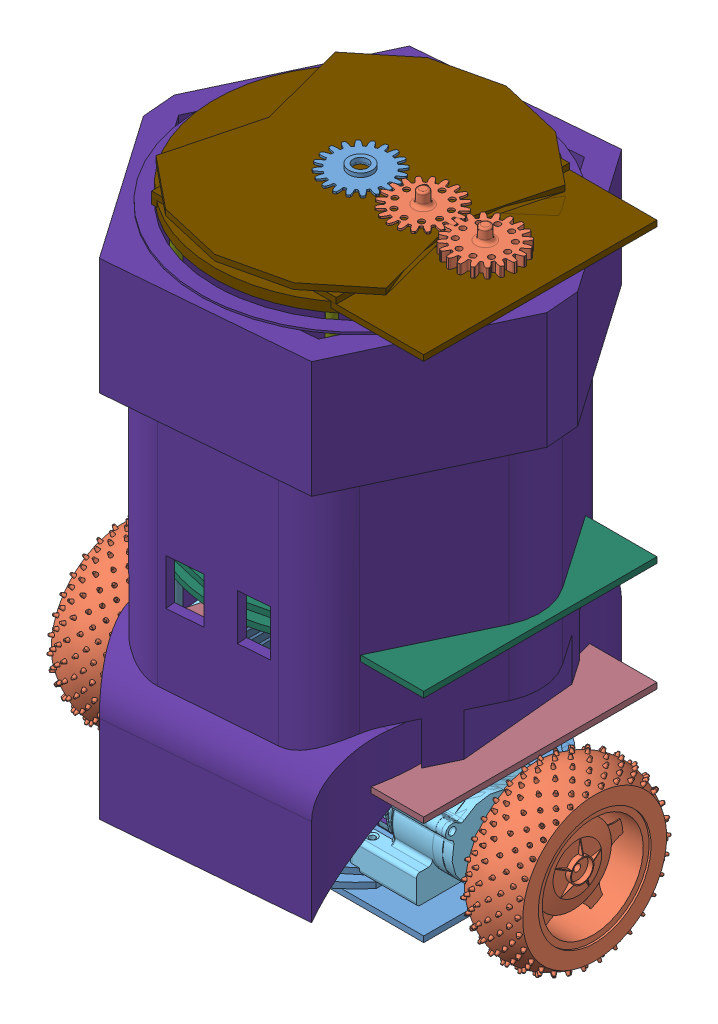
SolidWorks assembly Assembly_2, configuration Default. Lengths in mm.
Overall size (242.54 323.12 157.59).
45 component instances, 20 part files, 99 mates.
Components (placement in the parent):
- BASE PLATE COMPACT-1: BASE PLATE COMPACT [Default] at (9.1956 73.2306 176.3525) size (151.66 9 157.59)
- 85mm_Wheel-1: 85mm_Wheel [Default] at (-49.5434 86.804 117.1986) x (0 0.469219 0.883082) z (0 -0.883082 0.469219) size (89.76 30.03 89.76)
- Bearing_large-1: Bearing_large [Default] at (149.0346 86.804 117.1064) x (0 0.302035 0.953297) z (-1 0 0) size (34 34 10)
- Bearing_Modifiable-1: Bearing_Modifiable [Default] at (-9.2134 86.804 117.1986) x (0 0 -1) z (1 0 0) size (16 16 5)
- Gear Box Covering - Modifiable-1: Gear Box Covering - Modifiable [Default] at (122.6046 86.804 117.1064) x (0 -0.541121 -0.840945) z (1 0 0) size (87.3 57.46 46.55)
- Gear_Driven - LARGE-1: Gear_Driven - LARGE [Default] at (132.5346 86.804 117.1064) x (0 -0.920513 -0.390712) z (1 0 0) size (41.92 41.92 47.93)
- Gear_Driver-1: Gear_Driver [Default] at (129.4046 103.2 142.587) x (0 0.064546 -0.997915) z (1 0 0) size (21.81 21.81 25.3)
- IG32 MOTORS-1: IG32 MOTORS [Default] at (112.6046 103.2 142.587) x (-1 0 0) z (0 0 1) size (92 51.5 40)
- LINE SENSOR-1: LINE SENSOR [Default] at (106.6956 76.2306 130.3525) x (-1 0 0) z (0 0 1) size (100 13.5 28)
- Motor Driver-1: Motor Driver [Default] at (55.9629 132.2306 73.8421) size (71 27 36.5)
- Motor_Main_Shaft-1: Motor_Main_Shaft [Default] at (112.6046 103.2 142.587) x (0 -0.924225 0.381849) z (1 0 0) size (6 6 15)
- Gear Box Covering - Modifiable-2: Gear Box Covering - Modifiable [Default] at (-9.2134 86.804 117.1986) x (0 -0.541121 0.840945) z (-1 0 0) size (87.3 57.46 46.55)
- IG32 MOTORS-2: IG32 MOTORS [Default] at (0.7866 103.2 91.718) size (92 51.5 40)
- Motor_Main_Shaft-2: Motor_Main_Shaft [Default] at (-14.2134 103.2 91.718) x (0 0 -1) z (1 0 0) size (6 6 15)
- Gear_Driver-2: Gear_Driver [Default] at (-16.0134 103.2 91.718) x (0 0.135257 0.99081) z (-1 0 0) size (21.81 21.81 25.3)
- Gear_Driven - LARGE-2: Gear_Driven - LARGE [Default] at (-19.1434 86.804 117.1986) x (0 0.469219 0.883082) z (-1 0 0) size (41.92 41.92 47.93)
- Bearing_Modifiable-2: Bearing_Modifiable [Default] at (139.0346 103.2 142.587) x (0 -0.922949 -0.384923) z (1 0 0) size (16 16 5)
- Bearing_Modifiable-3: Bearing_Modifiable [Default] at (-30.6434 103.2 91.718) x (0 0.129255 -0.991611) z (1 0 0) size (16 16 5)
- Bearing_Modifiable-4: Bearing_Modifiable [Default] at (122.6046 86.804 117.1064) x (0 0.011286 0.999936) z (-1 0 0) size (16 16 5)
- Bearing_large-2: Bearing_large [Default] at (-35.6434 86.804 117.1986) x (0 0 -1) z (1 0 0) size (34 34 10)
- 85mm_Wheel-2: 85mm_Wheel [Default] at (162.9346 86.804 117.1064) x (0 -0.12189 -0.992544) z (0 -0.992544 0.12189) size (89.76 30.03 89.76)
- 4cm_spacers-1: 4cm_spacers [Default] at (96.6956 129.2306 61.5025) x (0.827993 0 0.560738) z (0 -1 0) size (5 5 55)
- 4cm_spacers-2: 4cm_spacers [Default] at (96.6956 129.2306 171.2025) x (0.889434 0 0.457064) z (0 -1 0) size (5 5 55)
- 4cm_spacers-3: 4cm_spacers [Default] at (16.6956 129.2306 171.2025) x (0.138561 0 0.990354) z (0 -1 0) size (5 5 55)
- 4cm_spacers-4: 4cm_spacers [Default] at (16.6956 129.2306 61.5025) x (0.594628 0 -0.804001) z (0 -1 0) size (5 5 55)
- Floor_Plates1-1: Floor_Plates1 [Default] at (9.1956 126.2306 176.3525) size (151.66 9 157.59)
- Motor Driver-2: Motor Driver [Default] at (60.9961 132.2306 157.7845) size (71 27 36.5)
- 3cm_spacers-1: 3cm_spacers [Default] at (96.6956 192.2306 171.2025) x (1 0 0) z (0 -1 0) size (5 5 55)
- 3cm_spacers-2: 3cm_spacers [Default] at (16.6956 192.2306 171.2025) x (1 0 0) z (0 -1 0) size (5 5 55)
- 3cm_spacers-3: 3cm_spacers [Default] at (16.6956 192.2306 61.5025) x (1 0 0) z (0 -1 0) size (5 5 55)
- 3cm_spacers-4: 3cm_spacers [Default] at (96.6956 192.2306 61.5025) x (1 0 0) z (0 -1 0) size (5 5 55)
- Floor_Plates2-1: Floor_Plates2 [Default] at (9.1956 182.2306 176.3525) size (151.66 9 150)
- 6cm_spacers-1: 6cm_spacers [Default] at (96.6956 330.2306 61.5025) x (1 0 0) z (0 -1 0) size (5 5 150)
- 6cm_spacers-2: 6cm_spacers [Default] at (96.6956 330.2306 171.2025) x (1 0 0) z (0 -1 0) size (5 5 150)
- 6cm_spacers-3: 6cm_spacers [Default] at (16.6956 330.2306 171.2025) x (1 0 0) z (0 -1 0) size (5 5 150)
- 6cm_spacers-4: 6cm_spacers [Default] at (16.6956 330.2306 61.5025) x (1 0 0) z (0 -1 0) size (5 5 150)
- Hex_Cover-1: Hex_Cover [Default] at (56.6956 76.2306 116.3525) x (0.996418 0 -0.084559) z (0.084559 0 0.996418) size (192.07 251 175) (hidden)
- Floor_Plates3-1: Floor_Plates3 [Default] at (9.1956 332.2306 176.3525) size (167.5 11 150)
- Bearing_Modifiable-5: Bearing_Modifiable [Default] at (56.6956 335.2306 116.3525) x (0.129255 0 -0.991611) z (0 -1 0) size (16 16 5)
- Bearing_Modifiable-8: Bearing_Modifiable [Default] at (56.6956 190.2306 116.3525) x (0.129255 0 -0.991611) z (0 -1 0) size (16 16 5)
- Gear_1-1: Gear_1 [Default] at (56.6956 339.7306 116.3525) x (0.837835 0 0.545924) z (0 -1 0) size (34.9 34.9 9)
- Bearing_Modifiable-9: Bearing_Modifiable [Default] at (120.8956 335.2306 116.3525) x (0.129255 0 -0.991611) z (0 -1 0) size (16 16 5)
- Bearing_Modifiable-10: Bearing_Modifiable [Default] at (88.8956 335.2306 116.3525) x (0.129255 0 -0.991611) z (0 -1 0) size (16 16 5)
- Gear_2-1: Gear_2 [Default] at (120.8956 339.7306 116.3525) x (0.836558 0 0.547878) z (0 1 0) size (34.9 34.9 19)
- Gear_2-2: Gear_2 [Default] at (88.8956 339.7306 116.3525) x (0.978484 0 0.206323) z (0 1 0) size (34.9 34.9 19)
Mates (geometry in assembly coordinates):
- BasePlate_&_LineSensor: coincident anti-aligned: plane of BASE PLATE COMPACT-1 through (127.509 76.2306 116.3525) normal (0 -1 0); plane of LINE SENSOR-1 through (106.6956 76.2306 130.3525) normal (0 1 0)
- Potentiometer&BasePlate: parallel anti-aligned: plane of BASE PLATE COMPACT-1 through (29.6956 84.2306 121.8525) normal (-1 0 0); plane of LINE SENSOR-1 through (28.6956 81.2306 120.8525) normal (1 0 0)
- LineSensor&BasePlate: concentric anti-aligned: cylinder of BASE PLATE COMPACT-1 through (9.1956 84.2306 127.8525) axis (0 -1 0) radius 1.711; cylinder of LINE SENSOR-1 through (9.1956 74.2306 127.8525) axis (0 1 0) radius 1.5
- BasePlate&GearBox1: concentric aligned: cylinder of BASE PLATE COMPACT-1 through (4.0366 68.2306 132.1499) axis (0 1 0) radius 1.75; cylinder of Gear Box Covering - Modifiable-2 through (4.0366 67.8227 132.1499) axis (0 1 0) radius 1.75
- Coincident14: coincident anti-aligned: plane of BASE PLATE COMPACT-1 through (127.509 79.2306 116.3525) normal (0 1 0); plane of Gear Box Covering - Modifiable-2 through (-24.2134 79.2306 117.1986) normal (0 -1 0)
- GearBox&BasePlate1: parallel anti-aligned: plane of BASE PLATE COMPACT-1 through (-2.4644 76.2306 70.2538) normal (-1 0 0); plane of Gear Box Covering - Modifiable-2 through (-4.2134 103.2 91.718) normal (1 0 0)
- BasePlate&GearBox2: concentric aligned: cylinder of BASE PLATE COMPACT-1 through (109.3546 68.2306 102.1551) axis (0 1 0) radius 1.75; cylinder of Gear Box Covering - Modifiable-1 through (109.3546 67.8227 102.1551) axis (0 1 0) radius 1.75
- GearBox&BasePlate2: parallel anti-aligned: plane of BASE PLATE COMPACT-1 through (115.8556 76.2306 70.2538) normal (1 0 0); plane of Gear Box Covering - Modifiable-1 through (117.6046 103.2 142.587) normal (-1 0 0)
- BasePlate&GearBox2C: coincident anti-aligned: plane of BASE PLATE COMPACT-1 through (127.509 79.2306 116.3525) normal (0 1 0); plane of Gear Box Covering - Modifiable-1 through (137.6046 79.2306 117.1064) normal (0 -1 0)
- MotorShaft&GearBox2: concentric aligned: cylinder of IG32 MOTORS-1 through (115.6046 103.2 142.587) axis (-1 0 0) radius 7.5; cylinder of Motor_Main_Shaft-1 through (127.6046 103.2 142.587) axis (-1 0 0) radius 3
- Motor&MotorShaft2: coincident anti-aligned: plane of IG32 MOTORS-1 through (112.6046 103.2 142.587) normal (1 0 0); plane of Motor_Main_Shaft-1 through (112.6046 103.2 142.587) normal (-1 0 0)
- Motor&MotorShaft1: concentric anti-aligned: cylinder of IG32 MOTORS-2 through (-2.2134 103.2 91.718) axis (1 0 0) radius 7.5; cylinder of Motor_Main_Shaft-2 through (0.7866 103.2 91.718) axis (-1 0 0) radius 3
- Motor&MotorShaft11: coincident anti-aligned: plane of IG32 MOTORS-2 through (0.7866 103.2 91.718) normal (-1 0 0); plane of Motor_Main_Shaft-2 through (0.7866 103.2 91.718) normal (1 0 0)
- Motor&GearBox1: concentric aligned: cylinder of Gear Box Covering - Modifiable-2 through (-14.2134 103.2 91.718) axis (1 0 0) radius 10.75; cylinder of IG32 MOTORS-2 through (-2.2134 103.2 91.718) axis (1 0 0) radius 10.5
- Motor&GearBox2: concentric aligned: cylinder of Gear Box Covering - Modifiable-1 through (127.6046 103.2 142.587) axis (-1 0 0) radius 10.75; cylinder of IG32 MOTORS-1 through (115.6046 103.2 142.587) axis (-1 0 0) radius 10.5
- MotorHole&GearBox2: concentric aligned: cylinder of Gear Box Covering - Modifiable-1 through (117.6046 116.7 142.587) axis (1 0 0) radius 1.75; cylinder of IG32 MOTORS-1 through (109.6046 116.7 142.587) axis (1 0 0) radius 1.5
- MotorHole&GearBox1: concentric aligned: cylinder of Gear Box Covering - Modifiable-2 through (-4.2134 116.7 91.718) axis (-1 0 0) radius 1.75; cylinder of IG32 MOTORS-2 through (3.7866 116.7 91.718) axis (-1 0 0) radius 1.5
- Motor2&GearBox2: coincident anti-aligned: plane of Gear Box Covering - Modifiable-2 through (0.7866 103.2 91.718) normal (1 0 0); plane of IG32 MOTORS-2 through (0.7866 103.2 91.718) normal (-1 0 0)
- Motor1&GearBox1: coincident anti-aligned: plane of Gear Box Covering - Modifiable-1 through (112.6046 103.2 142.587) normal (-1 0 0); plane of IG32 MOTORS-1 through (112.6046 103.2 142.587) normal (1 0 0)
- Concentric17: concentric aligned: cylinder of Motor_Main_Shaft-2 through (0.7866 103.2 91.718) axis (-1 0 0) radius 3; cone of Gear_Driver-2 through (-4.2114 103.2 91.718) axis (-1 0 0)
- Coincident25: coincident anti-aligned: plane of Motor_Main_Shaft-2 through (-14.2134 103.2 91.718) normal (-1 0 0); plane of Gear_Driver-2 through (-14.2134 103.2 91.718) normal (1 0 0)
- Concentric18: concentric anti-aligned: cylinder of Gear_Driver-2 through (-16.5134 103.2 91.718) axis (-1 0 0) radius 2.8; cylinder of Bearing_Modifiable-3 through (-30.6434 103.2 91.718) axis (1 0 0) radius 8
- Coincident26: coincident aligned: plane of Gear Box Covering - Modifiable-2 through (-30.6434 109.5417 71.6985) normal (-1 0 0); plane of Bearing_Modifiable-3 through (-30.6434 103.2 91.718) normal (-1 0 0)
- Concentric20: concentric anti-aligned: cylinder of Gear_Driver-1 through (115.4046 103.2 142.587) axis (1 0 0) radius 5.75; cylinder of Motor_Main_Shaft-1 through (127.6046 103.2 142.587) axis (-1 0 0) radius 3
- Coincident27: coincident anti-aligned: plane of Gear_Driver-1 through (127.6046 103.2 142.587) normal (-1 0 0); plane of Motor_Main_Shaft-1 through (127.6046 103.2 142.587) normal (1 0 0)
- Concentric22: concentric aligned: cylinder of Gear_Driver-1 through (129.9046 103.2 142.587) axis (1 0 0) radius 2.8; cylinder of Bearing_Modifiable-2 through (139.0346 103.2 142.587) axis (1 0 0) radius 8
- Coincident28: coincident aligned: plane of Gear Box Covering - Modifiable-1 through (144.0346 109.5417 162.6066) normal (1 0 0); plane of Bearing_Modifiable-2 through (144.0346 103.2 142.587) normal (1 0 0)
- Concentric23: concentric anti-aligned: cylinder of Bearing_Modifiable-1 through (-9.2134 86.804 117.1986) axis (1 0 0) radius 8; cylinder of Gear Box Covering - Modifiable-2 through (-4.2134 86.804 117.1986) axis (-1 0 0) radius 8.75
- Coincident29: coincident aligned: plane of Bearing_Modifiable-1 through (-9.2134 86.804 117.1986) normal (-1 0 0); plane of Gear Box Covering - Modifiable-2 through (-9.2134 103.2 91.718) normal (-1 0 0)
- Concentric24: concentric anti-aligned: cylinder of Gear Box Covering - Modifiable-1 through (117.6046 86.804 117.1064) axis (1 0 0) radius 8.75; cylinder of Bearing_Modifiable-4 through (122.6046 86.804 117.1064) axis (-1 0 0) radius 8
- Coincident30: coincident aligned: plane of Gear Box Covering - Modifiable-1 through (122.6046 103.2 142.587) normal (1 0 0); plane of Bearing_Modifiable-4 through (122.6046 86.804 117.1064) normal (1 0 0)
- Concentric25: concentric aligned: cylinder of Bearing_Modifiable-1 through (-4.2134 86.804 117.1986) axis (-1 0 0) radius 3; cylinder of Gear_Driven - LARGE-2 through (-4.2134 86.804 117.1986) axis (-1 0 0) radius 2.8
- Coincident31: coincident anti-aligned: plane of Gear Box Covering - Modifiable-2 through (-4.2134 86.804 117.1986) normal (-1 0 0); plane of Gear_Driven - LARGE-2 through (-4.2134 86.804 117.1986) normal (1 0 0)
- Concentric26: concentric aligned: cylinder of Gear_Driven - LARGE-1 through (117.6046 86.804 117.1064) axis (1 0 0) radius 2.8; cylinder of Bearing_Modifiable-4 through (117.6046 86.804 117.1064) axis (1 0 0) radius 3
- Coincident32: coincident anti-aligned: plane of Gear Box Covering - Modifiable-1 through (117.6046 86.804 117.1064) normal (1 0 0); plane of Gear_Driven - LARGE-1 through (117.6046 86.804 117.1064) normal (-1 0 0)
- Concentric27: concentric anti-aligned: cylinder of Gear_Driven - LARGE-2 through (-47.9434 86.804 117.1986) axis (1 0 0) radius 7.5; cylinder of Bearing_large-2 through (-25.6434 86.804 117.1986) axis (-1 0 0) radius 7.5
- Concentric28: concentric anti-aligned: cylinder of Bearing_large-1 through (139.0346 86.804 117.1064) axis (1 0 0) radius 7.5; cylinder of Gear_Driven - LARGE-1 through (161.3346 86.804 117.1064) axis (-1 0 0) radius 7.5
- Coincident33: coincident aligned: plane of Gear Box Covering - Modifiable-2 through (-35.6434 86.804 117.1986) normal (-1 0 0); plane of Bearing_large-2 through (-35.6434 86.804 117.1986) normal (-1 0 0)
- Coincident34: coincident aligned: plane of Bearing_large-1 through (149.0346 86.804 117.1064) normal (1 0 0); plane of Gear Box Covering - Modifiable-1 through (149.0346 86.804 117.1064) normal (1 0 0)
- Concentric29: concentric anti-aligned: cylinder of 85mm_Wheel-1 through (-47.9434 86.804 117.1986) axis (-1 0 0) radius 8.5; cylinder of Gear_Driven - LARGE-2 through (-47.9434 86.804 117.1986) axis (1 0 0) radius 7.5
- Parallel1: parallel aligned: plane of 85mm_Wheel-1 through (-47.9434 92.6969 120.8833) normal (0 -0.469219 -0.883082); plane of Gear_Driven - LARGE-2 through (-52.1434 87.0485 110.253) normal (0 -0.469219 -0.883082)
- Coincident39: coincident anti-aligned: plane of 85mm_Wheel-1 through (-52.1434 86.804 117.1986) normal (1 0 0); plane of Gear_Driven - LARGE-2 through (-52.1434 86.804 117.1986) normal (-1 0 0)
- Concentric30: concentric anti-aligned: cylinder of Gear_Driven - LARGE-1 through (161.3346 86.804 117.1064) axis (-1 0 0) radius 7.5; cylinder of 85mm_Wheel-2 through (161.3346 86.804 117.1064) axis (1 0 0) radius 8.5
- Coincident41: coincident anti-aligned: plane of Gear_Driven - LARGE-1 through (165.5346 89.5194 110.7088) normal (0 0.798623 -0.601832); plane of 85mm_Wheel-2 through (161.3346 93.7022 116.2593) normal (0 -0.798623 0.601832)
- Coincident42: coincident anti-aligned: plane of Gear_Driven - LARGE-1 through (165.5346 86.804 117.1064) normal (1 0 0); plane of 85mm_Wheel-2 through (165.5346 86.804 117.1064) normal (-1 0 0)
- Concentric31: concentric anti-aligned: cylinder of BASE PLATE COMPACT-1 through (96.6956 86.2306 61.5025) axis (0 -1 0) radius 1.25; cylinder of 4cm_spacers-1 through (96.6956 74.2306 61.5025) axis (0 1 0) radius 1.25
- Coincident43: coincident anti-aligned: plane of BASE PLATE COMPACT-1 through (127.509 79.2306 116.3525) normal (0 1 0); plane of 4cm_spacers-1 through (96.6956 79.2306 61.5025) normal (0 -1 0)
- Concentric32: concentric anti-aligned: cylinder of BASE PLATE COMPACT-1 through (16.6956 86.2306 61.5025) axis (0 -1 0) radius 1.25; cylinder of 4cm_spacers-4 through (16.6956 74.2306 61.5025) axis (0 1 0) radius 1.25
- Concentric33: concentric anti-aligned: cylinder of BASE PLATE COMPACT-1 through (16.6956 86.2306 171.2025) axis (0 -1 0) radius 1.25; cylinder of 4cm_spacers-3 through (16.6956 74.2306 171.2025) axis (0 1 0) radius 1.25
- Concentric34: concentric anti-aligned: cylinder of BASE PLATE COMPACT-1 through (96.6956 86.2306 171.2025) axis (0 -1 0) radius 1.25; cylinder of 4cm_spacers-2 through (96.6956 74.2306 171.2025) axis (0 1 0) radius 1.25
- Coincident44: coincident anti-aligned: plane of BASE PLATE COMPACT-1 through (127.509 79.2306 116.3525) normal (0 1 0); plane of 4cm_spacers-4 through (16.6956 79.2306 61.5025) normal (0 -1 0)
- Coincident45: coincident anti-aligned: plane of BASE PLATE COMPACT-1 through (127.509 79.2306 116.3525) normal (0 1 0); circle of 4cm_spacers-3
- Coincident46: coincident anti-aligned: plane of BASE PLATE COMPACT-1 through (127.509 79.2306 116.3525) normal (0 1 0); plane of 4cm_spacers-2 through (96.6956 79.2306 171.2025) normal (0 -1 0)
- Concentric35: concentric anti-aligned: cylinder of 4cm_spacers-4 through (16.6956 124.2306 61.5025) axis (0 1 0) radius 1.25; cylinder of Floor_Plates1-1 through (16.6956 139.2306 61.5025) axis (0 -1 0) radius 1.25
- Concentric36: concentric anti-aligned: line of 4cm_spacers-2 through (96.6956 124.2306 171.2025) axis (0 1 0); axis of Floor_Plates1-1 through (96.6956 132.2306 171.2025) axis (0 -1 0)
- Coincident47: coincident anti-aligned: plane of 4cm_spacers-1 through (96.6956 129.2306 61.5025) normal (0 1 0); plane of Floor_Plates1-1 through (127.509 129.2306 116.3525) normal (0 -1 0)
- Coincident48: coincident anti-aligned: plane of Floor_Plates1-1 through (127.509 132.2306 116.3525) normal (0 1 0); plane of Motor Driver-2 through (60.9961 132.2306 157.7845) normal (0 -1 0)
- Coincident49: coincident anti-aligned: plane of Motor Driver-1 through (55.9629 132.2306 73.8421) normal (0 -1 0); plane of Floor_Plates1-1 through (127.509 132.2306 116.3525) normal (0 1 0)
- Concentric37: concentric anti-aligned: cylinder of Floor_Plates1-1 through (16.6956 139.2306 171.2025) axis (0 -1 0) radius 1.25; cylinder of 3cm_spacers-2 through (16.6956 127.2306 171.2025) axis (0 1 0) radius 1.25
- Concentric38: concentric anti-aligned: cylinder of Floor_Plates1-1 through (16.6956 139.2306 61.5025) axis (0 -1 0) radius 1.25; cylinder of 3cm_spacers-3 through (16.6956 127.2306 61.5025) axis (0 1 0) radius 1.25
- Concentric39: concentric anti-aligned: cylinder of Floor_Plates1-1 through (96.6956 139.2306 171.2025) axis (0 -1 0) radius 1.25; cylinder of 3cm_spacers-1 through (96.6956 127.2306 171.2025) axis (0 1 0) radius 1.25
- Concentric40: concentric anti-aligned: cylinder of Floor_Plates1-1 through (96.6956 139.2306 61.5025) axis (0 -1 0) radius 1.25; cylinder of 3cm_spacers-4 through (96.6956 127.2306 61.5025) axis (0 1 0) radius 1.25
- Coincident50: coincident anti-aligned: plane of Floor_Plates1-1 through (127.509 132.2306 116.3525) normal (0 1 0); plane of 3cm_spacers-2 through (16.6956 132.2306 171.2025) normal (0 -1 0)
- Coincident52: coincident anti-aligned: plane of Floor_Plates1-1 through (127.509 132.2306 116.3525) normal (0 1 0); plane of 3cm_spacers-1 through (96.6956 132.2306 171.2025) normal (0 -1 0)
- Coincident53: coincident anti-aligned: plane of Floor_Plates1-1 through (127.509 132.2306 116.3525) normal (0 1 0); plane of 3cm_spacers-3 through (16.6956 132.2306 61.5025) normal (0 -1 0)
- Coincident54: coincident anti-aligned: plane of Floor_Plates1-1 through (127.509 132.2306 116.3525) normal (0 1 0); plane of 3cm_spacers-4 through (96.6956 132.2306 61.5025) normal (0 -1 0)
- Concentric41: concentric: cylinder of 3cm_spacers-3 through (16.6956 157.2306 61.5025) axis (0 1 0) radius 1.25; cylinder of Floor_Plates2-1 through (16.6956 175.2306 61.5025) axis (0 -1 0) radius 1.25
- Concentric42: concentric: cylinder of 3cm_spacers-1 through (96.6956 157.2306 171.2025) axis (0 1 0) radius 1.25; cylinder of Floor_Plates2-1 through (96.6956 175.2306 171.2025) axis (0 -1 0) radius 1.25
- Coincident55: coincident anti-aligned: plane of 3cm_spacers-3 through (16.6956 182.2306 61.5025) normal (0 1 0); plane of Floor_Plates2-1 through (56.6956 182.2306 116.3525) normal (0 -1 0)
- Concentric43: concentric: cylinder of Floor_Plates2-1 through (16.6956 175.2306 61.5025) axis (0 -1 0) radius 1.25; cylinder of 6cm_spacers-4 through (16.6956 160.2306 61.5025) axis (0 1 0) radius 1.25
- Concentric44: concentric: cylinder of Floor_Plates2-1 through (16.6956 175.2306 171.2025) axis (0 -1 0) radius 1.25; cylinder of 6cm_spacers-3 through (16.6956 160.2306 171.2025) axis (0 1 0) radius 1.25
- Concentric45: concentric: cylinder of Floor_Plates2-1 through (96.6956 175.2306 171.2025) axis (0 -1 0) radius 1.25; cylinder of 6cm_spacers-2 through (96.6956 160.2306 171.2025) axis (0 1 0) radius 1.25
- Concentric46: concentric: cylinder of Floor_Plates2-1 through (96.6956 175.2306 61.5025) axis (0 -1 0) radius 1.25; cylinder of 6cm_spacers-1 through (96.6956 160.2306 61.5025) axis (0 1 0) radius 1.25
- Coincident56: coincident anti-aligned: plane of Floor_Plates2-1 through (56.6956 185.2306 116.3525) normal (0 1 0); plane of 6cm_spacers-4 through (16.6956 185.2306 61.5025) normal (0 -1 0)
- Coincident58: coincident anti-aligned: plane of Floor_Plates2-1 through (56.6956 185.2306 116.3525) normal (0 1 0); plane of 6cm_spacers-1 through (96.6956 185.2306 61.5025) normal (0 -1 0)
- Coincident59: coincident anti-aligned: plane of Floor_Plates2-1 through (56.6956 185.2306 116.3525) normal (0 1 0); plane of 6cm_spacers-3 through (16.6956 185.2306 171.2025) normal (0 -1 0)
- Coincident60: coincident anti-aligned: plane of Floor_Plates2-1 through (56.6956 185.2306 116.3525) normal (0 1 0); plane of 6cm_spacers-2 through (96.6956 185.2306 171.2025) normal (0 -1 0)
- Coincident64: coincident: plane of BASE PLATE COMPACT-1 through (127.509 76.2306 116.3525) normal (0 -1 0); plane of Hex_Cover-1 through (56.6956 76.2306 116.3525) normal (0 -1 0)
- Concentric47: concentric anti-aligned: cylinder of 6cm_spacers-3 through (16.6956 185.2306 171.2025) axis (0 1 0) radius 2.5; cylinder of Floor_Plates3-1 through (16.6956 345.2306 171.2025) axis (0 -1 0) radius 1.25
- Concentric48: concentric anti-aligned: cylinder of 6cm_spacers-2 through (96.6956 185.2306 171.2025) axis (0 1 0) radius 2.5; cylinder of Floor_Plates3-1 through (96.6956 345.2306 171.2025) axis (0 -1 0) radius 1.25
- Coincident65: coincident anti-aligned: plane of 6cm_spacers-3 through (16.6956 330.2306 171.2025) normal (0 1 0); plane of Floor_Plates3-1 through (56.6956 330.2306 116.3525) normal (0 -1 0)
- Concentric49: concentric anti-aligned: cylinder of Floor_Plates3-1 through (56.6956 325.2306 116.3525) axis (0 1 0) radius 8.5; cylinder of Bearing_Modifiable-5 through (56.6956 335.2306 116.3525) axis (0 -1 0) radius 8
- Coincident66: coincident aligned: plane of Floor_Plates3-1 through (56.6956 335.2306 116.3525) normal (0 1 0); plane of Bearing_Modifiable-5 through (56.6956 335.2306 116.3525) normal (0 1 0)
- Concentric52: concentric aligned: cylinder of Floor_Plates2-1 through (56.6956 190.2306 116.3525) axis (0 -1 0) radius 8.35; cylinder of Bearing_Modifiable-8 through (56.6956 190.2306 116.3525) axis (0 -1 0) radius 8
- Coincident69: coincident anti-aligned: plane of Floor_Plates2-1 through (56.6956 190.2306 116.3525) normal (0 1 0); circle of Bearing_Modifiable-8
- Concentric53: concentric: cylinder of Bearing_Modifiable-5 through (56.6956 285.2306 116.3525) axis (0 1 0) radius 3; cylinder of Gear_1-1 through (56.6956 299.2306 116.3525) axis (0 -1 0) radius 3.8
- Coincident70: coincident: plane of Floor_Plates3-1 through (56.6956 290.2306 116.3525) normal (0 1 0); plane of Gear_1-1 through (56.6956 290.2306 116.3525) normal (0 -1 0)
- Concentric56: concentric aligned: cylinder of Bearing_Modifiable-5 through (56.6956 330.2306 116.3525) axis (0 1 0) radius 3; cylinder of Gear_1-1 through (56.6956 335.2306 116.3525) axis (0 1 0) radius 3.8
- Coincident76: coincident anti-aligned: plane of Bearing_Modifiable-5 through (56.6956 335.2306 116.3525) normal (0 1 0); plane of Gear_1-1 through (56.6956 335.2306 116.3525) normal (0 -1 0)
- Concentric58: concentric anti-aligned: cylinder of Floor_Plates3-1 through (120.8956 325.2306 116.3525) axis (0 1 0) radius 8.5; cylinder of Bearing_Modifiable-9 through (120.8956 335.2306 116.3525) axis (0 -1 0) radius 8
- Concentric59: concentric anti-aligned: cylinder of Floor_Plates3-1 through (88.8956 325.2306 116.3525) axis (0 1 0) radius 8.5; cylinder of Bearing_Modifiable-10 through (88.8956 335.2306 116.3525) axis (0 -1 0) radius 8
- Coincident77: coincident aligned: plane of Floor_Plates3-1 through (56.6956 335.2306 116.3525) normal (0 1 0); plane of Bearing_Modifiable-10 through (88.8956 335.2306 116.3525) normal (0 1 0)
- Coincident78: coincident aligned: plane of Floor_Plates3-1 through (56.6956 335.2306 116.3525) normal (0 1 0); plane of Bearing_Modifiable-9 through (120.8956 335.2306 116.3525) normal (0 1 0)
- Concentric60: concentric anti-aligned: cylinder of Bearing_Modifiable-10 through (88.8956 330.2306 116.3525) axis (0 1 0) radius 3; cylinder of Gear_2-2 through (88.8956 349.2306 116.3525) axis (0 -1 0) radius 2.85
- Concentric61: concentric anti-aligned: cylinder of Bearing_Modifiable-9 through (120.8956 330.2306 116.3525) axis (0 1 0) radius 3; cylinder of Gear_2-1 through (120.8956 349.2306 116.3525) axis (0 -1 0) radius 2.85
- Coincident79: coincident aligned: plane of Floor_Plates3-1 through (56.6956 330.2306 116.3525) normal (0 -1 0); circle of Gear_2-1
- Coincident80: coincident aligned: plane of Floor_Plates3-1 through (56.6956 330.2306 116.3525) normal (0 -1 0); circle of Gear_2-2
- GearMate1: gear = 36 : 35.2 mm: cylinder of Gear_1-1 through (56.6956 292.2306 116.3525) axis (0 1 0) radius 17.6; cylinder of Gear_2-2 through (88.8956 297.2306 116.3525) axis (0 -1 0) radius 17.6
- GearMate2: gear = 35.2 : 35.2 mm: cylinder of Gear_2-2 through (88.8956 297.2306 116.3525) axis (0 -1 0) radius 17.6; cylinder of Gear_2-1 through (120.8956 297.2306 116.3525) axis (0 -1 0) radius 17.6
